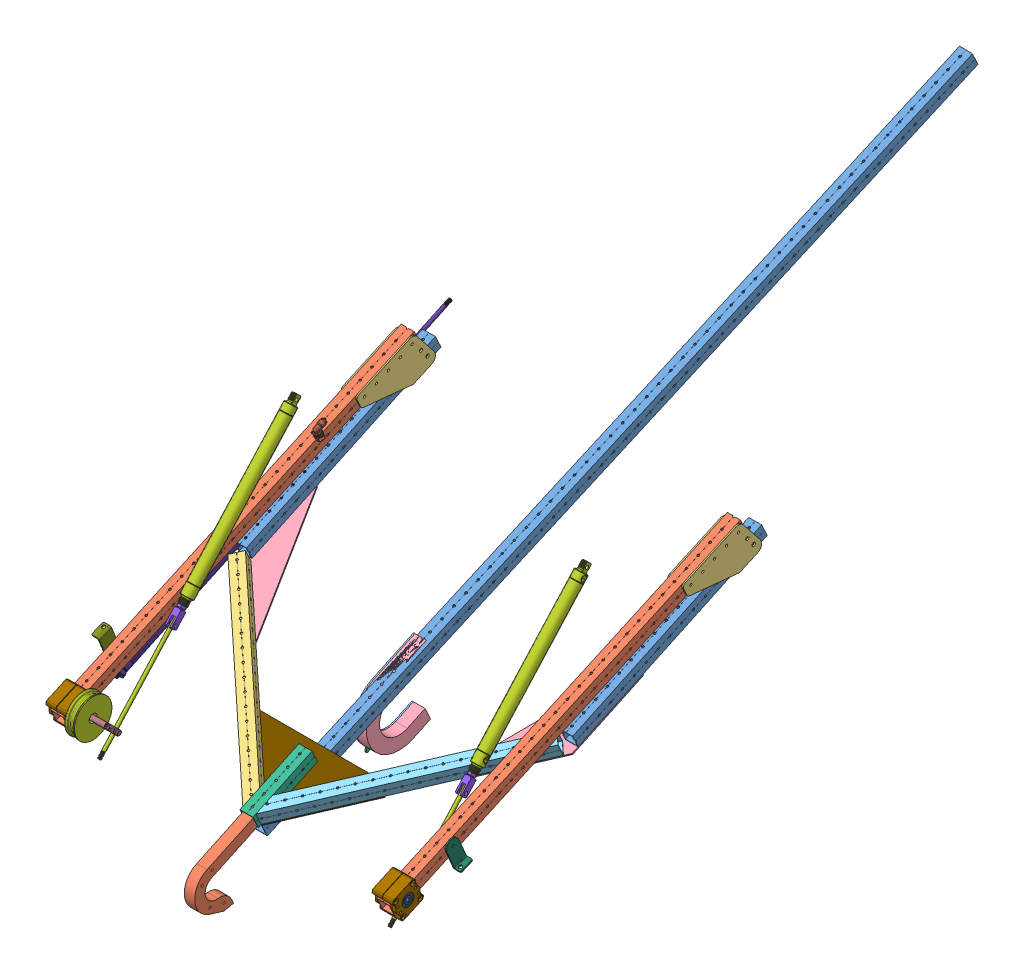
SolidWorks assembly 1250-20-CLMB, configuration Default. Lengths in mm.
Overall size (812.8 3037.02 3006.16).
46 component instances, 28 part files, 88 mates.
Components (placement in the parent):
- Climber-1: Climber [Default] x (1 0 0) z (0 0 -1) size (0 3037.02 3006.16)
- 1250-20-D9003-1: 1250-20-D9003 [Default] at (317.5 -531.061 282.2991) x (0 -0.905553 -0.424234) z (0 0.424234 -0.905553) size (25.4 25.4 406.4)
- 1250-20-D9002-1: 1250-20-D9002 [Default] at (317.5 -184.1192 -354.7001) x (0 -0.911038 -0.412323) z (0 -0.412323 0.911038) size (25.4 25.4 749.27)
- LinkPlate0001-2: LinkPlate0001 [Default] at (330.2 -184.1329 -354.6697) x (0 -0.412323 0.911038) z (0 0.911038 0.412323) size (254 2.54 76.29)
- 1250-20-D9002-2: 1250-20-D9002 [Default] at (-317.5 -184.1192 -354.7001) x (0 0.911038 0.412323) z (0 -0.412323 0.911038) size (25.4 25.4 749.27)
- 1250-20-D9003-3: 1250-20-D9003 [Default] at (-317.5 -531.061 282.2991) x (0 0.905553 0.424234) z (0 0.424234 -0.905553) size (25.4 25.4 406.4)
- LinkPlate0001-5: LinkPlate0001 [Default] at (-332.74 -184.1329 -354.6697) x (0 -0.412323 0.911038) z (0 0.911038 0.412323) size (254 2.54 76.29)
- HookAssem-12: HookAssem [Default] at (0 -483.9972 -3.7668) x (0 -0.905553 -0.424234) z (0 0.424234 -0.905553) size (127 33.02 152.4) (hidden)
  - middlepart2-1: middlepart2 [Default] at origin size (127 22.86 152.4)
  - hook-1: hook [Default] at (0 11.43 0) size (127 2.54 152.4)
  - Part2^HookAssem-1: Part2^HookAssem [Default] at origin (virtual)
  - Part3^HookAssem-1: Part3^HookAssem [Default] at origin (virtual)
  - Hook2-1: Hook2 [Default] at (38.3482 13.97 -44.376) x (0.75166 0 -0.659551) z (0.659551 0 0.75166) size (130.96 2.54 12.7)
  - hook-2: hook [Default] at (0 -13.97 0) size (127 2.54 152.4)
  - Hook2-2: Hook2 [Default] at (38.3482 -16.51 -44.376) x (0.75166 0 -0.659551) z (0.659551 0 0.75166) size (130.96 2.54 12.7)
- 6498K403_ROUND BODY AIR CYLINDER-1: 6498K403_ROUND BODY AIR CYLINDER [6498K403] at (282.575 -268.1391 17.0979) x (0 0.741197 -0.671288) z (1 0 0) size (572.84 21.84 21.84)
- Air cylinder Clevis-1: Air cylinder Clevis [Default] at (282.575 -386.0865 123.9206) x (-1 0 0) z (0 0.671288 0.741197) size (14.66 35.92 12.7)
- 6498K403_ROUND BODY AIR CYLINDER-2: 6498K403_ROUND BODY AIR CYLINDER [6498K403] at (-282.575 -268.1391 17.0979) x (0 0.741197 -0.671288) z (-1 0 0) size (572.84 21.84 21.84)
- Air cylinder Clevis-2: Air cylinder Clevis [Default] at (-282.575 -386.0865 123.9206) x (-1 0 0) z (0 0.671288 0.741197) size (14.66 35.92 12.7)
- LinkPlate0001-6: LinkPlate0001 [Default] at (302.26 -184.1329 -354.6697) x (0 -0.412323 0.911038) z (0 0.911038 0.412323) size (254 2.54 76.29)
- LinkPlate0001-7: LinkPlate0001 [Default] at (-304.8 -184.1329 -354.6697) x (0 -0.412323 0.911038) z (0 0.911038 0.412323) size (254 2.54 76.29)
- 217-5852-2: 217-5852 [Default] at (327.55 -482.6 304.8) x (0 0.412323 -0.911038) z (1 0 0) size (50.97 48.1 23.6)
- 217-5852-3: 217-5852 [Default] at (307.45 -482.6 304.8) x (0 -0.412323 0.911038) z (-1 0 0) size (50.97 48.1 23.6)
- 6383K214_BALL BEARING-1: 6383K214_BALL BEARING [6383K214] at (301.625 -482.6 304.8) x (0 0.339591 -0.940573) z (-1 0 0) size (25.4 25.4 7.95)
- 6383K214_BALL BEARING-2: 6383K214_BALL BEARING [6383K214] at (333.375 -482.6 304.8) x (0 0.570317 -0.821425) z (1 0 0) size (25.4 25.4 7.95)
- 217-5852-6: 217-5852 [Default] at (-307.45 -482.6 304.8) x (0 -0.412323 0.911038) z (1 0 0) size (50.97 48.1 23.6)
- 217-5852-8: 217-5852 [Default] at (-327.55 -482.6 304.8) x (0 0.412323 -0.911038) z (-1 0 0) size (50.97 48.1 23.6)
- 5779K152_PUSH-TO-CONNECT TUBE FITTING FOR AIR-1: 5779K152_PUSH-TO-CONNECT TUBE FITTING FOR AIR [5779K152] at (-260.985 -217.3032 -123.454) x (1 0 0) z (0 -0.906308 -0.422618) size (14.31 26.12 26.64)
- Bearings-1: Bearings [217-2733] at (-297.5382 -482.6 304.8) x (0 0.986676 0.162695) z (-1 0 0) size (24.61 24.61 7.11)
- Bearings-2: Bearings [217-2733] at (-337.4618 -482.6 304.8) x (0 -0.956721 0.291007) z (1 0 0) size (24.61 24.61 7.11)
- 90201A339_EXTREME-STRENGTH GRADE 9 STEEL CAP SCREW-1: 90201A339_EXTREME-STRENGTH GRADE 9 STEEL CAP SCREW [90201A339] at (-284.8997 -482.6 304.8) size (122.04 16.5 14.29)
- 90107A127_TYPE 316 STAINLESS STEEL FLAT WASHER-1: 90107A127_TYPE 316 STAINLESS STEEL FLAT WASHER [90107A127] at (-337.4618 -482.6 304.8) x (0 0.603999 -0.796985) z (0 0.796985 0.603999) size (19.05 1.02 19.05)
- 1250-20-D9008-1: 1250-20-D9008 [Default] at (332.74 -481.5577 181.0226) x (0 0.392559 -0.919727) z (1 0 0) size (25.4 52.62 14.52)
- 1250-20-D9006-2: 1250-20-D9006 [Default] at (-332.74 -388.9052 219.8809) x (0 0.381529 -0.924357) z (-1 0 0) size (25.4 52.62 14.52)
- 6498K642_ROUND BODY AIR CYLINDER-1: 6498K642_ROUND BODY AIR CYLINDER [6498K642] at (-338.3651 -403.932 12.6514) x (0 -0.421819 0.90668) z (0 -0.90668 -0.421819) size (725.24 27.5 23.81)
- Air cylinder Clevis-3: Air cylinder Clevis [Default] at (-338.3651 -300.9329 -208.7402) x (1 0 0) z (0 0.90668 0.421819) size (14.66 35.92 12.7)
- 1250-20-D9009-1: 1250-20-D9009 [Default] at (12.7 -539.4739 264.3333) x (-1 0 0) z (0 0.424234 -0.905553) size (276.85 2.54 143.68)
- 1250-20-D9010-1: 1250-20-D9010 [Default] at (13.0651 -233.1453 -419.4802) x (0 -0.905553 -0.424234) z (0.017737 0.424167 -0.90541) size (25.4 25.4 1498.6) (hidden)
- 1250-20-CLAW-1: 1250-20-CLAW [Default] at (-10.16 -464.3548 384.553) x (1 0 0) z (0 -0.905553 -0.424234) size (20.32 245.11 96.52)
- 1250-20-D9013-1: 1250-20-D9013 [Default] at (217.5956 -615.753 463.0792) x (0 0.905553 0.424234) z (-0.707107 0.299978 -0.640322) size (25.4 25.4 436.31)
- 1250-20-D9012-1: 1250-20-D9012 [Default] at (222.4369 -450.4964 74.4054) x (-0.707107 0.299978 -0.640322) z (0.707107 0.299978 -0.640322) size (125.72 2.54 260.16)
- 1250-20-D9011-3: 1250-20-D9011 [Default] at (-217.5956 -615.753 463.0792) x (0 0.905553 0.424234) z (0.707107 0.299978 -0.640322) size (25.4 25.4 436.31)
- 1250-20-D9012-2: 1250-20-D9012 [Default] at (-222.4369 -448.1963 75.483) x (0.707107 0.299978 -0.640322) z (-0.707107 0.299978 -0.640322) size (125.72 2.54 260.16)
- 1250-20-D9014-1: 1250-20-D9014 [Default] at (0 -210.435 -402.0968) x (0 0.905553 0.424234) z (0 0.424234 -0.905553) size (25.4 25.4 127)
- 6498K642_ROUND BODY AIR CYLINDER-2: 6498K642_ROUND BODY AIR CYLINDER [6498K642] at (-338.3651 -403.932 12.6514) x (0 -0.421819 0.90668) z (0 -0.90668 -0.421819) size (725.24 27.5 23.81)
- 1250-20-D9015-1: 1250-20-D9015 [Default] at (-297.5382 -482.6 304.8) x (1 0 0) z (0 -0.157692 -0.987488) size (18.98 73.03 73.03)
Mates (geometry in assembly coordinates):
- Coincident41: coincident: plane of Climber-1 through (0 0 0) normal (1 0 0); plane of assembly through (0 0 0) normal (1 0 0)
- Coincident50: coincident: plane of 1250-20-D9003-1 through (317.5 -531.061 282.2991) normal (0 -0.905553 -0.424234); plane of 1250-20-D9003-3 through (-317.5 -531.061 282.2991) normal (0 0.905553 0.424234)
- Coincident53: coincident: plane of 1250-20-D9003-1 through (317.5 -531.061 282.2991) normal (0 0.424234 -0.905553); plane of 1250-20-D9003-3 through (-317.5 -531.061 282.2991) normal (0 0.424234 -0.905553)
- Coincident61: coincident: plane of Climber-1 through (0 0 0) normal (0 0 -1); plane of assembly through (0 0 0) normal (0 0 1)
- Distance20: distance = 317.5 mm: plane of assembly through (0 0 0) normal (1 0 0); plane of 1250-20-D9003-1 through (317.5 -531.061 282.2991) normal (-1 0 0)
- Coincident83: coincident: plane of Climber-1 through (0 0 0) normal (0 -1 0); plane of assembly through (0 0 0) normal (0 1 0)
- Coincident84: coincident: plane of 1250-20-D9003-1 through (317.5 -531.061 282.2991) normal (0 -0.905553 -0.424234); line of Climber-1 through (0 -213.1828 -396.2316) axis (0 -0.424234 0.905553)
- Coincident86: coincident: plane of 1250-20-D9003-3 through (-317.5 -213.1828 -396.2316) normal (0 0.424234 -0.905553); point of Climber-1
- Coincident92: coincident: point of Climber-1; line of 1250-20-D9002-1 through (303.848 -482.6 304.8) axis (1 0 0)
- Coincident94: coincident: plane of 1250-20-D9003-1 through (304.8 -201.6822 -390.8438) normal (-1 0 0); plane of 1250-20-D9002-1 through (304.8 -481.5028 333.1769) normal (-1 0 0)
- Coincident95: coincident: plane of 1250-20-D9002-1 through (304.8 -481.5028 333.1769) normal (0 0.911038 0.412323); plane of LinkPlate0001-2 through (332.74 -224.9278 -233.7314) normal (0 0.911038 0.412323)
- Coincident96: coincident: plane of 1250-20-D9002-1 through (330.2 -481.5028 333.1769) normal (1 0 0); plane of LinkPlate0001-2 through (330.2 -230.4949 -375.6525) normal (-1 0 0)
- Coincident97: coincident: plane of 1250-20-D9002-1 through (317.5 -184.1329 -354.6697) normal (0 -0.412323 0.911038); plane of LinkPlate0001-2 through (330.2 -184.1329 -354.6697) normal (0 -0.412323 0.911038)
- Coincident98: coincident: plane of 1250-20-D9002-2 through (-304.8 -481.5028 333.1769) normal (0 0.911038 0.412323); plane of LinkPlate0001-5 through (-330.2 -224.9278 -233.7314) normal (0 0.911038 0.412323)
- Coincident99: coincident: plane of 1250-20-D9002-2 through (-317.5 -184.1329 -354.6697) normal (0 -0.412323 0.911038); plane of LinkPlate0001-5 through (-332.74 -184.1329 -354.6697) normal (0 -0.412323 0.911038)
- Coincident100: coincident: plane of 1250-20-D9002-2 through (-330.2 -504.6432 322.7038) normal (-1 0 0); plane of LinkPlate0001-5 through (-330.2 -230.4949 -375.6525) normal (1 0 0)
- Width6: width: plane of 1250-20-D9003-1 through (330.2 -201.6822 -390.8438) normal (1 0 0); plane of 1250-20-D9003-3 through (-330.2 -224.6833 -401.6193) normal (-1 0 0); plane of HookAssem-12/hook-2 through (13.97 -483.9972 -3.7668) normal (1 0 0); plane of HookAssem-12/hook-1 through (-13.97 -483.9972 -3.7668) normal (-1 0 0)
- Concentric1: concentric: point of Climber-1; cylinder of 6498K403_ROUND BODY AIR CYLINDER-1 through (274.6375 -146.05 -93.476) axis (1 0 0) radius 3.175
- Parallel12: parallel: plane of 6498K403_ROUND BODY AIR CYLINDER-1 through (287.401 -147.1226 -81.7955) normal (1 0 0); plane of assembly through (0 0 0) normal (1 0 0)
- Coincident150: coincident: line of Climber-1 through (0 -407.7368 143.529) axis (0 0.741197 -0.671288); plane of 6498K403_ROUND BODY AIR CYLINDER-1 through (282.575 -268.1391 17.0979) normal (0 0.671288 0.741197)
- Coincident151: coincident: plane of 6498K403_ROUND BODY AIR CYLINDER-1 through (282.575 -386.0865 123.9206) normal (0 -0.741197 0.671288); plane of Air cylinder Clevis-1 through (282.575 -377.5611 133.3338) normal (0 0.741197 -0.671288)
- Concentric2: concentric: cylinder of 6498K403_ROUND BODY AIR CYLINDER-1 through (282.575 -376.6733 115.3953) axis (0 -0.741197 0.671288) radius 10.922; circle of Air cylinder Clevis-1
- Distance26: distance = 15.875 mm: plane of Air cylinder Clevis-1 through (288.925 -385.7774 132.2079) normal (1 0 0); plane of 1250-20-D9002-1 through (304.8 -481.5028 333.1769) normal (-1 0 0)
- Coincident153: coincident: plane of 6498K403_ROUND BODY AIR CYLINDER-1 through (282.575 -268.1391 17.0979) normal (0 0.671288 0.741197); plane of 6498K403_ROUND BODY AIR CYLINDER-2 through (-282.575 -268.1391 17.0979) normal (0 -0.671288 -0.741197)
- Symmetric1: symmetric: plane of 6498K403_ROUND BODY AIR CYLINDER-1 through (282.575 -268.1391 17.0979) normal (1 0 0); plane of 6498K403_ROUND BODY AIR CYLINDER-2 through (-282.575 -268.1391 17.0979) normal (-1 0 0); plane of assembly
- Coincident154: coincident: plane of 6498K403_ROUND BODY AIR CYLINDER-1 through (282.575 -268.1391 17.0979) normal (0 0.741197 -0.671288); plane of 6498K403_ROUND BODY AIR CYLINDER-2 through (-282.575 -268.1391 17.0979) normal (0 0.741197 -0.671288)
- Coincident155: coincident: plane of 6498K403_ROUND BODY AIR CYLINDER-2 through (-282.575 -386.0865 123.9206) normal (0 -0.741197 0.671288); plane of Air cylinder Clevis-2 through (-282.575 -377.5611 133.3338) normal (0 0.741197 -0.671288)
- Coincident156: coincident: plane of Air cylinder Clevis-1 through (288.925 -416.7061 143.085) normal (0 -0.671288 -0.741197); plane of Air cylinder Clevis-2 through (-276.225 -416.7061 143.085) normal (0 -0.671288 -0.741197)
- Symmetric2: symmetric: plane of 1250-20-D9003-1 through (304.8 -201.6822 -390.8438) normal (-1 0 0); plane of 1250-20-D9003-3 through (-304.8 -224.6833 -401.6193) normal (1 0 0); plane of assembly
- Coincident173: coincident: plane of 1250-20-D9003-1 through (304.8 -201.6822 -390.8438) normal (-1 0 0); plane of LinkPlate0001-6 through (304.8 -230.4949 -375.6525) normal (1 0 0)
- Coincident174: coincident: plane of LinkPlate0001-2 through (330.2 -184.1329 -354.6697) normal (0 -0.412323 0.911038); plane of LinkPlate0001-6 through (302.26 -184.1329 -354.6697) normal (0 -0.412323 0.911038)
- Coincident175: coincident: plane of LinkPlate0001-2 through (330.2 -184.1329 -354.6697) normal (0 0.911038 0.412323); plane of LinkPlate0001-6 through (302.26 -184.1329 -354.6697) normal (0 0.911038 0.412323)
- Coincident176: coincident: plane of LinkPlate0001-5 through (-332.74 -184.1329 -354.6697) normal (0 0.911038 0.412323); plane of LinkPlate0001-7 through (-304.8 -184.1329 -354.6697) normal (0 0.911038 0.412323)
- Coincident177: coincident: plane of LinkPlate0001-5 through (-332.74 -184.1329 -354.6697) normal (0 -0.412323 0.911038); plane of LinkPlate0001-7 through (-304.8 -184.1329 -354.6697) normal (0 -0.412323 0.911038)
- Parallel48: parallel: plane of LinkPlate0001-5 through (-330.2 -224.9278 -233.7314) normal (0 0.911038 0.412323); plane of LinkPlate0001-7 through (-302.26 -224.9278 -233.7314) normal (0 0.911038 0.412323)
- Concentric5: concentric: cylinder of 1250-20-D9002-1 through (304.8 -482.6 304.8) axis (1 0 0) radius 6.731; cylinder of 217-5852-2 through (337.55 -482.6 304.8) axis (-1 0 0) radius 11.1125
- Parallel17: parallel: plane of 1250-20-D9002-1 through (304.8 -504.6432 322.7038) normal (0 -0.911038 -0.412323); plane of 217-5852-2 through (388.7689 -483.7203 276.4127) normal (0 0.911038 0.412323)
- Coincident184: coincident: plane of 1250-20-D9002-1 through (330.2 -481.5028 333.1769) normal (1 0 0); plane of 217-5852-2 through (330.2 -482.6 304.8) normal (-1 0 0)
- Concentric6: concentric: cylinder of 217-5852-3 through (297.45 -482.6 304.8) axis (1 0 0) radius 11.1125; cylinder of 217-5852-2 through (337.55 -482.6 304.8) axis (-1 0 0) radius 11.1125
- Coincident187: coincident: plane of 1250-20-D9002-1 through (304.8 -481.5028 333.1769) normal (-1 0 0); plane of 217-5852-3 through (304.8 -482.6 304.8) normal (1 0 0)
- Parallel22: parallel: plane of 217-5852-2 through (337.55 -514.7671 318.1219) normal (0.012217 -0.91097 -0.412293); plane of 217-5852-3 through (297.45 -450.4329 291.4781) normal (-0.012217 0.91097 0.412293)
- Concentric7: concentric: cylinder of 1250-20-D9002-1 through (304.8 -482.6 304.8) axis (1 0 0) radius 6.731; cylinder of 6383K214_BALL BEARING-1 through (298.45 -482.6 304.8) axis (-1 0 0) radius 6.7437
- Coincident189: coincident: plane of 1250-20-D9002-1 through (304.8 -481.5028 333.1769) normal (-1 0 0); plane of 6383K214_BALL BEARING-1 through (304.8 -492.7535 301.1341) normal (1 0 0)
- Concentric9: concentric: cylinder of 1250-20-D9002-1 through (304.8 -482.6 304.8) axis (1 0 0) radius 6.731; cylinder of 6383K214_BALL BEARING-2 through (336.55 -482.6 304.8) axis (1 0 0) radius 6.7437
- Coincident191: coincident: plane of 1250-20-D9002-1 through (330.2 -481.5028 333.1769) normal (1 0 0); plane of 6383K214_BALL BEARING-2 through (330.2 -473.7327 310.9566) normal (-1 0 0)
- Coincident193: coincident: plane of 1250-20-D9002-2 through (-304.8 -504.6432 322.7038) normal (1 0 0); plane of 217-5852-6 through (-304.8 -482.6 304.8) normal (-1 0 0)
- Concentric14: concentric: cylinder of 1250-20-D9002-2 through (-304.8 -482.6 304.8) axis (-1 0 0) radius 6.731; cylinder of 217-5852-6 through (-297.45 -482.6 304.8) axis (-1 0 0) radius 11.1125
- Parallel42: parallel: plane of 1250-20-D9002-2 through (-304.8 -481.5028 333.1769) normal (0 0.911038 0.412323); plane of 217-5852-6 through (-246.2311 -481.4797 333.1873) normal (0 -0.911038 -0.412323)
- Concentric16: concentric: cylinder of 217-5852-6 through (-297.45 -482.6 304.8) axis (-1 0 0) radius 11.1125; cylinder of 217-5852-8 through (-337.55 -482.6 304.8) axis (1 0 0) radius 11.1125
- Coincident214: coincident: plane of 1250-20-D9002-2 through (-330.2 -504.6432 322.7038) normal (-1 0 0); plane of 217-5852-8 through (-330.2 -482.6 304.8) normal (1 0 0)
- Parallel43: parallel: plane of 217-5852-6 through (-297.45 -450.4329 291.4781) normal (0.012217 0.91097 0.412293); plane of 217-5852-8 through (-337.55 -514.7671 318.1219) normal (-0.012217 -0.91097 -0.412293)
- Coincident241: coincident: plane of 1250-20-D9003-3 through (-304.8 -224.6833 -401.6193) normal (1 0 0); plane of LinkPlate0001-7 through (-304.8 -230.4949 -375.6525) normal (-1 0 0)
- Coincident2571: coincident: plane of 217-5852-6 through (-303.05 -482.6 304.8) normal (-1 0 0); plane of Bearings-1 through (-303.05 -482.6 304.8) normal (1 0 0)
- Concentric251: concentric: cylinder of 217-5852-8 through (-337.55 -482.6 304.8) axis (1 0 0) radius 11.1125; cylinder of Bearings-1 through (-297.5382 -482.6 304.8) axis (-1 0 0) radius 4.7625
- Coincident2581: coincident: plane of 217-5852-8 through (-331.95 -482.6 304.8) normal (1 0 0); plane of Bearings-2 through (-331.95 -482.6 304.8) normal (-1 0 0)
- Concentric261: concentric: cylinder of Bearings-1 through (-297.5382 -482.6 304.8) axis (-1 0 0) radius 4.7625; cylinder of Bearings-2 through (-337.4618 -482.6 304.8) axis (1 0 0) radius 4.7625
- Concentric271: concentric: cylinder of Bearings-2 through (-337.4618 -482.6 304.8) axis (1 0 0) radius 4.7625; cylinder of 90201A339_EXTREME-STRENGTH GRADE 9 STEEL CAP SCREW-1 through (-338.4778 -482.6 304.8) axis (1 0 0) radius 4.7625
- Concentric281: concentric: cylinder of 90201A339_EXTREME-STRENGTH GRADE 9 STEEL CAP SCREW-1 through (-338.4778 -482.6 304.8) axis (1 0 0) radius 4.7625; cylinder of 90107A127_TYPE 316 STAINLESS STEEL FLAT WASHER-1 through (-337.4618 -482.6 304.8) axis (-1 0 0) radius 5.1562
- Coincident2621: coincident: plane of Bearings-2 through (-337.4618 -482.6 304.8) normal (-1 0 0); plane of 90107A127_TYPE 316 STAINLESS STEEL FLAT WASHER-1 through (-337.4618 -482.6 304.8) normal (1 0 0)
- Coincident2631: coincident: plane of 90201A339_EXTREME-STRENGTH GRADE 9 STEEL CAP SCREW-1 through (-338.4778 -478.4756 311.9438) normal (1 0 0); plane of 90107A127_TYPE 316 STAINLESS STEEL FLAT WASHER-1 through (-338.4778 -482.6 304.8) normal (-1 0 0)
- Coincident2669: coincident: plane of 1250-20-D9002-1 through (330.2 -481.5028 333.1769) normal (1 0 0); plane of 1250-20-D9008-1 through (330.2 -481.5577 181.0226) normal (-1 0 0)
- Coincident2676: coincident: plane of 1250-20-D9002-2 through (-330.2 -504.6432 322.7038) normal (-1 0 0); plane of 1250-20-D9006-2 through (-330.2 -388.9052 219.8809) normal (1 0 0)
- Concentric293: concentric: cylinder of 1250-20-D9002-2 through (-304.8 -440.708 212.2386) axis (-1 0 0) radius 2.0701; cylinder of 1250-20-D9006-2 through (-330.2 -440.708 212.2386) axis (-1 0 0) radius 2.0701
- Coincident2701: coincident: plane of HookAssem-12/middlepart2-1 through (-11.43 -449.4957 12.3965) normal (0 -0.905553 -0.424234); plane of 1250-20-D9010-1 through (39.0535 73.0869 -1103.088) normal (0 -0.905553 -0.424234)
- Concentric299: concentric: cylinder of 1250-20-D9009-1 through (0 -534.0861 252.8328) axis (0 0.905553 0.424234) radius 2.0955; cylinder of 1250-20-D9010-1 through (0 -534.0861 252.8328) axis (0 -0.905553 -0.424234) radius 2.0701
- Coincident2702: coincident: plane of 1250-20-D9009-1 through (12.7 -539.4739 264.3333) normal (0 -0.905553 -0.424234); plane of 1250-20-D9010-1 through (39.0535 96.0879 -1092.3124) normal (0 0.905553 0.424234)
- Coincident2731: coincident: plane of 1250-20-D9009-1 through (12.7 -537.1738 265.4108) normal (0 0.905553 0.424234); plane of 1250-20-D9013-1 through (-321.2197 -406.2893 -13.9701) normal (0 -0.905553 -0.424234)
- Coincident2741: coincident: plane of 1250-20-D9003-1 through (330.2 -201.6822 -390.8438) normal (1 0 0); plane of 1250-20-D9012-1 through (330.2 -402.4796 -22.1022) normal (1 0 0)
- Coincident2742: coincident: plane of 1250-20-D9003-1 through (330.2 -224.6833 -401.6193) normal (0 -0.905553 -0.424234); plane of 1250-20-D9012-1 through (222.4369 -448.1963 75.483) normal (0 0.905553 0.424234)
- Coincident2744: coincident: plane of 1250-20-D9012-1 through (222.4369 -448.1963 75.483) normal (0.707107 -0.299978 0.640322); plane of 1250-20-D9011-3 through (321.2197 -406.2893 -13.9701) normal (0.707107 -0.299978 0.640322)
- Coincident2745: coincident: plane of 1250-20-D9012-1 through (222.4369 -448.1963 75.483) normal (0 0.905553 0.424234); plane of 1250-20-D9011-3 through (303.2592 -398.6699 -30.2343) normal (0 -0.905553 -0.424234)
- Coincident2751: coincident: plane of 1250-20-D9003-3 through (-330.2 -224.6833 -401.6193) normal (0 -0.905553 -0.424234); plane of 1250-20-D9012-2 through (-222.4369 -448.1963 75.483) normal (0 0.905553 0.424234)
- Coincident2752: coincident: plane of 1250-20-D9003-3 through (-330.2 -224.6833 -401.6193) normal (-1 0 0); plane of 1250-20-D9012-2 through (-330.2 -404.7797 -23.1797) normal (-1 0 0)
- Coincident2759: coincident: plane of 1250-20-D9013-1 through (-321.2197 -406.2893 -13.9701) normal (0 -0.905553 -0.424234); plane of 1250-20-D9012-2 through (-222.4369 -448.1963 75.483) normal (0 0.905553 0.424234)
- Coincident2760: coincident: plane of 1250-20-D9013-1 through (-321.2197 -406.2893 -13.9701) normal (-0.707107 -0.299978 0.640322); plane of 1250-20-D9012-2 through (-222.4369 -450.4964 74.4054) normal (-0.707107 -0.299978 0.640322)
- Distance39: distance = 12.7 mm: line of 1250-20-D9012-1 through (330.2 -402.4796 -22.1022) axis (0 -0.905553 -0.424234); plane of 1250-20-D9011-3 through (312.2395 -390.9791 -16.7144) normal (0.707107 0.299978 -0.640322)
- Distance40: distance = 12.7 mm: plane of 1250-20-D9013-1 through (-312.2395 -390.9791 -16.7144) normal (-0.707107 0.299978 -0.640322); line of 1250-20-D9012-2 through (-330.2 -404.7797 -23.1797) axis (0 0.905553 0.424234)
- Distance41: distance = 12.7 mm: plane of 1250-20-D9003-1 through (317.5 -385.5913 -28.2149) normal (0 -0.424234 0.905553); line of 1250-20-D9012-1 through (330.2 -402.4796 -22.1022) axis (0 -0.905553 -0.424234)
- Distance42: distance = 12.7 mm: line of 1250-20-D9012-2 through (-330.2 -404.7797 -23.1797) axis (0 0.905553 0.424234); plane of 1250-20-D9003-3 through (-317.5 -385.5913 -28.2149) normal (0 -0.424234 0.905553)
- Coincident2769: coincident: plane of 1250-20-D9009-1 through (12.7 -537.1738 265.4108) normal (0.707107 -0.299978 0.640322); plane of 1250-20-D9011-3 through (321.2197 -406.2893 -13.9701) normal (0.707107 -0.299978 0.640322)
- Coincident2770: coincident: plane of 1250-20-D9009-1 through (-12.7 -537.1738 265.4108) normal (-0.707107 -0.299978 0.640322); plane of 1250-20-D9013-1 through (-321.2197 -406.2893 -13.9701) normal (-0.707107 -0.299978 0.640322)
- Coincident2771: coincident: plane of 1250-20-D9011-3 through (303.2592 -398.6699 -30.2343) normal (0 -0.905553 -0.424234); plane of 1250-20-D9014-1 through (-12.7 95.9428 -1086.0153) normal (0 -0.905553 -0.424234)
- Width8: width: plane of 1250-20-D9014-1 through (11.684 107.4433 -1080.6275) normal (-1 0 0); plane of 1250-20-D9014-1 through (-11.684 107.4433 -1080.6275) normal (1 0 0); plane of 1250-20-CLAW-1 through (-10.16 -601.0314 350.8269) normal (-1 0 0); plane of 1250-20-CLAW-1 through (10.16 -601.0314 350.8269) normal (1 0 0)
- Concentric300: concentric: point of Climber-1; cylinder of 90201A339_EXTREME-STRENGTH GRADE 9 STEEL CAP SCREW-1 through (-338.4778 -482.6 304.8) axis (1 0 0) radius 4.7625
- Coincident2772: coincident: plane of 1250-20-D9002-2 through (-304.8 -504.6432 322.7038) normal (1 0 0); plane of LinkPlate0001-7 through (-304.8 -230.4949 -375.6525) normal (-1 0 0)
- Coincident2774: coincident: plane of 1250-20-D9002-1 through (317.5 -184.1192 -354.7001) normal (0 -0.911038 -0.412323); plane of 1250-20-D9002-2 through (-317.5 -184.1192 -354.7001) normal (0 0.911038 0.412323)
- Distance44: distance = 3.175 mm: plane of Bearings-1 through (-297.5382 -482.6 304.8) normal (1 0 0); plane of 1250-20-D9015-1 through (-294.3632 -490.4382 306.0517) normal (-1 0 0)
- Concentric302: concentric: cylinder of 90201A339_EXTREME-STRENGTH GRADE 9 STEEL CAP SCREW-1 through (-338.4778 -482.6 304.8) axis (1 0 0) radius 4.7625; cylinder of 1250-20-D9015-1 through (-319.6896 -482.6 304.8) axis (-1 0 0) radius 7.9375
